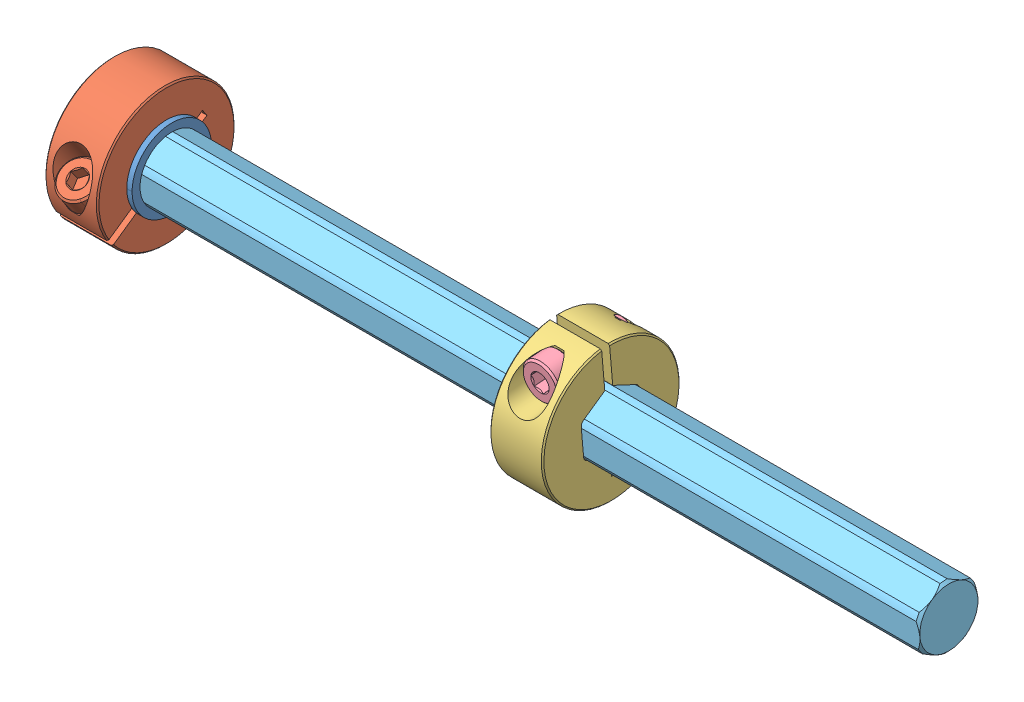
SolidWorks assembly Wheel On Axle, configuration Default. Lengths in mm.
Overall size (160 36.19 36.19).
7 component instances, 5 part files, 7 mates.
Components (placement in the parent):
- 12mm ID 1mm Thick Shim.step-1: 12mm ID 1mm Thick Shim.step [Default] at (96.3395 368.4088 360.6953) x (0 1 0) z (0 0 1) size (15 1 15)
- 12mm Axle Collar-1: 12mm Axle Collar [Default] at (108.8907 347.9293 346.8971) x (0 -0.819808 -0.572638) z (0 0.572638 -0.819808) size (26 10 25.98)
- 12mm ID 1mm Thick Shim.step-2: 12mm ID 1mm Thick Shim.step [Default] at (169.3395 368.4088 360.6953) x (0 0.9933 -0.115568) z (0 0.115568 0.9933) size (15 1 15)
- 12mm Axle Collar.STEP-1: 12mm Axle Collar.STEP [Default] at (155.7883 370.9464 336.132) x (0 0.086015 -0.996294) z (0 -0.996294 -0.086015) size (26 10 26.9)
  - 2910-1026-4012.STEP-1: 2910-1026-4012.STEP [Default] at (-24.6906 18.5512 0.4154) size (26 10 25.98)
  - 2800-0004-0012_90128A207.STEP-1: 2800-0004-0012_90128A207.STEP [Default] at (-16.4406 18.5512 -8.5319) x (0 0.713618 0.700535) z (1 0 0) size (7 7 16.01)
- 12mm REX 160mm-1: 12mm REX 160mm [Default] at (163.0395 368.4088 360.6953) x (0 -0.423656 -0.905823) z (0 -0.905823 0.423656) size (12 160 12.01)
Mates (geometry in assembly coordinates):
- Concentric1: concentric: circle of 12mm ID 1mm Thick Shim.step-1; circle of 12mm REX 160mm-1
- Coincident1: coincident: plane of 12mm Axle Collar.STEP-1/2910-1026-4012.STEP-1 through (164.5177 363.4267 363.0255) normal (0 0.905823 -0.423656); plane of 12mm REX 160mm-1 through (243.0395 363.4267 363.0255) normal (0 -0.905823 0.423656)
- Coincident2: coincident: plane of 12mm Axle Collar.STEP-1/2910-1026-4012.STEP-1 through (164.5177 368.8818 355.2157) normal (0 -0.086015 0.996294); plane of 12mm REX 160mm-1 through (243.0395 368.8818 355.2157) normal (0 0.086015 -0.996294)
- Coincident3: coincident: plane of 12mm ID 1mm Thick Shim.step-2 through (169.3395 368.4088 360.6953) normal (1 0 0); plane of 12mm Axle Collar.STEP-1/2910-1026-4012.STEP-1 through (169.3395 368.4088 360.6953) normal (-1 0 0)
- Coincident7: coincident: circle of 12mm ID 1mm Thick Shim.step-1; plane of 12mm Axle Collar-1 through (95.3395 368.4088 360.6953) normal (1 0 0)
- Coincident8: coincident: plane of 12mm Axle Collar-1 through (100.1613 373.3908 358.3652) normal (0 -0.905823 0.423656); plane of 12mm REX 160mm-1 through (243.0395 373.3908 358.3652) normal (0 0.905823 -0.423656)
- Coincident9: coincident: plane of 12mm Axle Collar-1 through (100.1613 372.9177 363.8449) normal (0 -0.819808 -0.572638); plane of 12mm REX 160mm-1 through (243.0395 372.9177 363.8449) normal (0 0.819808 0.572638)
